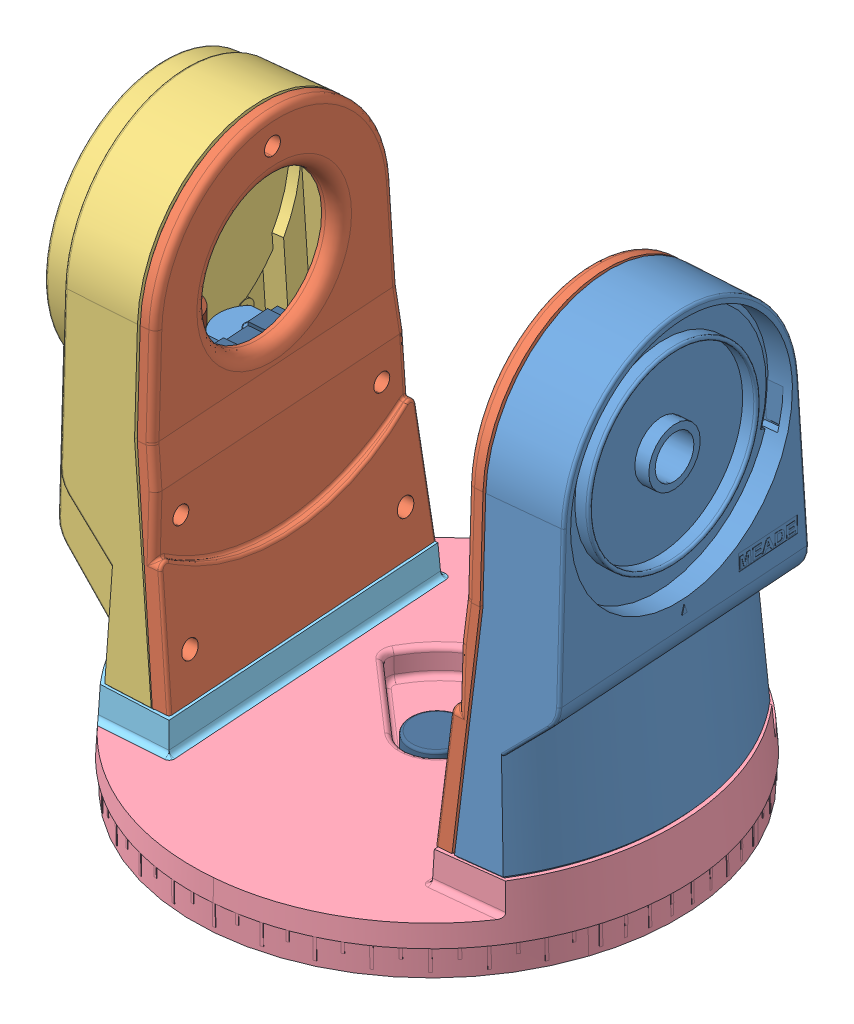
SolidWorks assembly fourche, configuration Défaut. Lengths in mm.
Overall size (198.85 238.33 188.61).
67 component instances, 42 part files, 82 mates.
Components (placement in the parent):
- branche equilibrage-1: branche equilibrage [Défaut] at (-444.0293 45.9192 -837.0232) x (0.999848 0.017413 0.00001) z (0.00001 -0.001172 0.999999) size (42.16 177.75 110.07)
- Plaque carter équilibrage-1: Plaque carter équilibrage [Défaut] at (-443.0317 45.9366 -837.0903) x (0.999848 0.017413 0.00001) z (0.00001 -0.001172 0.999999) size (27.56 165.18 109.18)
- Plaque carter équilibrage-2: Plaque carter équilibrage [Défaut] at (-468.0617 45.0668 -480.7137) x (-0.999848 -0.017413 -0.00001) z (-0.00001 0.001172 -0.999999) size (27.56 165.18 109.18)
- branche motorisée-1: branche motorisée [Défaut] at (-441.716 45.9434 -837.1795) x (0.999848 0.017413 0.00001) z (0.00001 -0.001172 0.999999) size (49.59 177.72 110.04)
- PIED DE fourche-1: PIED DE fourche [Défaut] at (-454.4692 -14.4541 -658.8869) x (0.999848 0.017413 0.00001) z (0.00001 -0.001172 0.999999) size (191.94 35.1 188.57)
  - Pied de fourche-1: Pied de fourche [Défaut] at (12.1809 59.9857 -178.2534) size (191.94 35.1 188.57)
  - Pied de fourche1-1: Pied de fourche1 [Défaut] at (-12.1809 59.9857 178.0188) x (-1 0 0) z (0 0 -1) size (54.8 35.1 115.86)
- rondelle vis m8_50-1: rondelle vis m8_50 [Défaut] at (-454.2843 -25.0712 -659.0167) x (0.997592 0.017452 -0.067129) z (0.017413 -0.999848 -0.001172) size (26.8 26.16 7)
- VisHM8_50-1: VisHM8_50 [Défaut] at (-454.3818 -19.4721 -659.0102) x (0.997592 0.017452 -0.067129) z (0.017413 -0.999848 -0.001172) size (12.6 14.55 55.47)
- limiteur de couple embase-1: limiteur de couple embase [Défaut] at (-453.5008 -70.0544 -659.0694) x (0.06714 0 0.997744) z (-0.997592 -0.017452 0.067129) size (25.3 5 25.3)
- Roue à denture hélicoïdale m=0,5 Z=60-1: Roue à denture hélicoïdale m=0,5 Z=60 [Défaut] at (-453.6431 -61.8856 -659.0599) x (0.201032 0.002353 0.979582) z (-0.017413 0.999848 0.001172) size (31.07 31.07 6.34)
- Levier de débrayage-1: Levier de débrayage [Défaut] at (-491.4971 43.1006 -833.8173) x (0.963244 0.01709 -0.268082) z (0.268062 0.003539 0.963395) size (36.12 10 38.96)
- plateau-1: plateau [Défaut] at (-454.3861 -19.2221 -659.0099) x (-0.997592 -0.017452 0.067129) z (0.017413 -0.999848 -0.001172) size (170 170 47)
- EcrouHM 20-2: EcrouHM 20 [Défaut] at (-453.9456 -44.5183 -659.0395) x (0.06714 0 0.997744) z (-0.017413 0.999848 0.001172) size (30 34.64 12)
- motoreducteur fourche-1: motoreducteur fourche [Défaut] at (-542.1299 45.8782 -641.824) x (0.06714 0 0.997744) z (0.997592 0.017452 -0.067129) size (70.5 139.71 33.06)
  - rep. 01 pignon arbre moteur + disque-1: rep. 01 pignon arbre moteur + disque [Défaut] at (0 -0.36 0) size (19 10.8 19)
  - rep. 02-03 roue Z56-1: rep. 02-03 roue Z56 [Défaut] at (0.8779 -0.6486 0.8082) x (0.995701 0 0.092628) z (-0.092628 0 0.995701) size (28.76 10.95 28.76)
  - rep. 08-09 roue inter-1: rep. 08-09 roue inter [Défaut] at (-0.15 -0.2381 0) x (1 0 0) z (0 0 1) size (12.96 5.74 12.96)
  - rep. 06-07 roue inter-1: rep. 06-07 roue inter [Défaut] at (-0.15 -0.0981 0) x (1 0 0) z (0 0 1) size (13 5.74 13)
  - rep. 04-05 roue inter-1: rep. 04-05 roue inter [Défaut] at (-21.6079 -0.6386 5.1059) x (0.907401 0 -0.420265) z (0.420265 0 0.907401) size (13 5.74 13)
  - bati-1: bati [Défaut] at (103.3128 129.885 -87.3106) size (70.5 138.91 24)
    - Axe Rep19bis-1: Axe Rep19bis [Défaut] at (-92.1856 -130.245 98.2871) x (-0.137137 0 0.990552) z (-0.990552 0 -0.137137) size (3 14 3)
    - moteur-1: moteur [Défaut] at (-103.3128 -129.885 87.3106) size (18 46.5 24)
    - axe-1: axe [Défaut] at (-111.605 -120.0821 97.7106) x (0.934599 0 -0.355704) z (0 -1 0) size (3 3 39)
    - bati2-1: bati2 [Défaut] at (-77.4849 -277.8736 138.6581) x (1 0 0) z (0 0 -1) size (17.4 55.11 17.4)
      - rondelle alu-1: rondelle alu [Défaut] at (-55.9783 -35.2009 30.6529) size (17.4 2.5 17.4)
      - Rondelle M6_1-1: Rondelle M6_1 [Défaut] at (-55.9783 -35.2009 30.6529) size (16.67 2.55 16.67)
      - rondelle alu_1-1: rondelle alu_1 [Défaut] at (-55.9783 -35.2009 30.6529) size (17.4 2.5 17.4)
      - Entretoise_1-1: Entretoise_1 [Défaut] at (-55.9783 -35.2009 30.6529) size (16.5 6 16.5)
      - Entretoise-1: Entretoise [Défaut] at (-55.9783 -35.2009 30.6529) size (16.5 6 16.5)
      - Rondelle M6-1: Rondelle M6 [Défaut] at (-55.9783 -35.2009 30.6529) size (16.67 2.55 16.67)
      - rep. 16 Ecrou M6-1: rep. 16 Ecrou M6 [Défaut] at (18.5294 -120.4752 48.0628) x (-0.896454 0 -0.443136) z (-0.443136 0 0.896454) size (12.68 6 11.39)
    - corps1-1: corps1 [Défaut] at (-126.5989 -147.7633 97.7106) size (62.7 74.5 12)
    - corps2-1: corps2 [Défaut] at (-126.5989 -147.7633 85.7106) size (62.7 50 12) (hidden)
    - châpe en alu-1: châpe en alu [Défaut] at (-133.4632 -157.3984 87.2051) size (33.3 38 19.61)
  - vis-1: vis [Défaut] at (7.3554 -71.4832 9.6533) x (1 0 0) z (0 1 0) size (33.09 33.06 82.71)
    - Vis san fin m=0,5 - 1 filet(s)-2: Vis san fin m=0,5 - 1 filet(s) [Défaut] at (-0.6479 -0.6412 0.3804) x (0.7262 -0.687484 0) z (0 0 1) size (8.16 8.16 68.9)
    - rep12-4: rep12 [Défaut] at (-11.6724 36.0347 43.7266) x (0.537117 -0.843508 0) z (-0.843508 -0.537117 0) size (23.91 29.81 24)
  - engrenage-1: engrenage [Défaut] at (-45.9983 -125.8694 31.0757) x (-0.919401 0 0.393321) z (0.393321 0 0.919401) size (12.99 17.44 12.99)
    - rep.11SLDPRT-1: rep.11SLDPRT [Défaut] at (-64.557 -106.8565 -14.5787) size (9.52 16 9.52)
    - rep. yacine-1: rep. yacine [Défaut] at (-64.557 -106.8565 -14.5787) size (12.99 1.44 12.99)
  - Vis à tête cylindrique à six pans creux Chc M2,5 - 8-1: Vis à tête cylindrique à six pans creux Chc M2,5 - 8 [Défaut] at (6.7074 -20.6971 10.2945) x (0.636786 0 0.771041) z (0 -1 0) size (4.2 4.2 10.57)
  - joint 9 5 emb-1: joint 9 5 emb [Défaut] at (6.7074 -89.1506 10.2945) size (13.5 2 13.5)
  - joint 9 5 emb-2: joint 9 5 emb [Défaut] at (6.7074 -53.1506 10.2945) size (13.5 2 13.5)
- Vis sans tête à six pans creux à bout cuvette M3 - 3-1: Vis sans tête à six pans creux à bout cuvette M3 - 3 [Réaliste] at (-445.1418 -17.1499 -659.6319) x (-0.019293 -0.859815 -0.51024) z (0.066624 -0.510307 0.857408) size (3.03 3.08 3.04)
- Vis à tête cylindrique bombée cruciforme type H M3 - 10-1: Vis à tête cylindrique bombée cruciforme type H M3 - 10 [Filetage Réaliste] at (-521.841 56.7793 -695.504) x (-0.997592 -0.017452 0.067129) z (-0.0364 0.955572 -0.292501) size (12.58 5.6 5.6)
- Vis à tête cylindrique bombée cruciforme type H M3 - 10-2: Vis à tête cylindrique bombée cruciforme type H M3 - 10 [Filetage Réaliste] at (-508.9533 16.8988 -611.179) x (-0.997592 -0.017452 0.067129) z (-0.040277 -0.642181 -0.765494) size (12.58 5.6 5.6)
- Vis à tête cylindrique bombée cruciforme type H M3 - 10-3: Vis à tête cylindrique bombée cruciforme type H M3 - 10 [Filetage Réaliste] at (-514.8616 16.8988 -698.9804) x (-0.997592 -0.017452 0.067129) z (-0.068087 0.06176 -0.995766) size (12.58 5.6 5.6)
- Vis à tête cylindrique bombée cruciforme type H M3 - 10-4: Vis à tête cylindrique bombée cruciforme type H M3 - 10 [Filetage Réaliste] at (-521.2936 154.7556 -654.4481) x (-0.997592 -0.017452 0.067129) z (-0.06714 0 -0.997744) size (12.58 5.6 5.6)
- Vis à tête cylindrique bombée cruciforme type H M3 - 10-5: Vis à tête cylindrique bombée cruciforme type H M3 - 10 [Filetage Réaliste] at (-516.3356 56.7793 -613.689) x (-0.997592 -0.017452 0.067129) z (-0.06714 0 -0.997744) size (12.58 5.6 5.6)
- Vis à tête cylindrique bombée cruciforme type H M3 - 10-7: Vis à tête cylindrique bombée cruciforme type H M3 - 10 [Filetage Réaliste] at (-393.6444 157.0051 -663.0973) x (0.997592 0.017452 -0.067129) z (0.06714 0 0.997744) size (12.58 5.6 5.6)
- Vis à tête cylindrique bombée cruciforme type H M3 - 10-8: Vis à tête cylindrique bombée cruciforme type H M3 - 10 [Filetage Réaliste] at (-401.1787 18.9039 -706.6898) x (0.997592 0.017452 -0.067129) z (0.06714 0 0.997744) size (12.58 5.6 5.6)
- Vis à tête cylindrique bombée cruciforme type H M3 - 10-10: Vis à tête cylindrique bombée cruciforme type H M3 - 10 [Filetage Réaliste] at (-395.1895 59.0113 -704.086) x (0.997592 0.017452 -0.067129) z (0.06714 0 0.997744) size (12.58 5.6 5.6)
- Vis à tête cylindrique fendue CS M4 - 10-1: Vis à tête cylindrique fendue CS M4 - 10 [Défaut] at (-539.7157 125.5672 -628.3483) x (0.067415 -0.016315 0.997592) z (-0.997592 -0.017452 0.067129) size (7 7 10.62)
- Vis à tête cylindrique fendue CS M4 - 10-2: Vis à tête cylindrique fendue CS M4 - 10 [Défaut] at (-538.2089 116.0774 -615.8713) x (0.067415 -0.016315 0.997592) z (-0.997592 -0.017452 0.067129) size (7 7 10.62)
- Vis à tête cylindrique fendue CS M4 - 10-3: Vis à tête cylindrique fendue CS M4 - 10 [Défaut] at (-539.3849 106.5701 -628.3705) x (0.067415 -0.016315 0.997592) z (-0.997592 -0.017452 0.067129) size (7 7 10.62)
- Vis à tête cylindrique bombée cruciforme type H M3 - 12-2: Vis à tête cylindrique bombée cruciforme type H M3 - 12 [Filetage Réaliste] at (-395.2704 18.9039 -618.8883) x (0.997592 0.017452 -0.067129) z (0.067129 0.000586 0.997744) size (14.59 5.6 5.6)
- Vis à tête cylindrique bombée cruciforme type H M3 - 12-3: Vis à tête cylindrique bombée cruciforme type H M3 - 12 [Filetage Réaliste] at (-389.684 59.0113 -622.271) x (0.997592 0.017452 -0.067129) z (0.068185 -0.42423 0.902984) size (14.59 5.6 5.6)
- Vis à tête cylindrique bombée cruciforme type H M3 - 25-1: Vis à tête cylindrique bombée cruciforme type H M3 - 25 [Filetage Réaliste] at (-516.5693 58.6063 -628.1014) x (-0.997592 -0.017452 0.067129) z (-0.067129 0.486457 -0.871122) size (32.61 5.6 5.6)
- Vis à tête cylindrique bombée cruciforme type H M3 - 25-2: Vis à tête cylindrique bombée cruciforme type H M3 - 25 [Filetage Réaliste] at (-520.3322 72.7741 -680.3366) x (-0.997592 -0.017452 0.067129) z (-0.067129 0.486457 -0.871122) size (32.61 5.6 5.6)
- Vis à tête cylindrique bombée cruciforme type H M3 - 25-3: Vis à tête cylindrique bombée cruciforme type H M3 - 25 [Filetage Réaliste] at (-519.8272 43.7786 -680.3706) x (-0.997592 -0.017452 0.067129) z (0.067053 0.00493 0.997737) size (32.61 5.6 5.6)
- Vis à tête cylindrique bombée cruciforme type H M3 - 20-1: Vis à tête cylindrique bombée cruciforme type H M3 - 20 [Filetage Réaliste] at (-531.1265 -25.9655 -653.8459) x (-0.017413 0.999848 0.001172) z (0.998816 0.017342 0.045444) size (22.61 5.6 5.6)
- Vis à tête cylindrique bombée cruciforme type H M3 - 20-2: Vis à tête cylindrique bombée cruciforme type H M3 - 20 [Filetage Réaliste] at (-512.8439 -25.695 -612.9812) x (-0.017413 0.999848 0.001172) z (0.998816 0.017342 0.045444) size (22.61 5.6 5.6)
- Vis à tête cylindrique bombée cruciforme type H M3 - 20-3: Vis à tête cylindrique bombée cruciforme type H M3 - 20 [Filetage Réaliste] at (-517.7505 -25.6821 -696.841) x (-0.017413 0.999848 0.001172) z (0.998816 0.017342 0.045444) size (22.61 5.6 5.6)
- Vis à tête cylindrique bombée cruciforme type H M3 - 20-4: Vis à tête cylindrique bombée cruciforme type H M3 - 20 [Filetage Réaliste] at (-395.7403 -23.5476 -705.0512) x (-0.017413 0.999848 0.001172) z (0.998816 0.017342 0.045444) size (22.61 5.6 5.6)
- Vis à tête cylindrique bombée cruciforme type H M3 - 20-5: Vis à tête cylindrique bombée cruciforme type H M3 - 20 [Filetage Réaliste] at (-377.4577 -23.2771 -664.1865) x (-0.017413 0.999848 0.001172) z (0.998816 0.017342 0.045444) size (22.61 5.6 5.6)
- Vis à tête cylindrique bombée cruciforme type H M3 - 20-6: Vis à tête cylindrique bombée cruciforme type H M3 - 20 [Filetage Réaliste] at (-390.8337 -23.5604 -621.1914) x (-0.017413 0.999848 0.001172) z (0.998816 0.017342 0.045444) size (22.61 5.6 5.6)
Mates (geometry in assembly coordinates):
- Coïncidente2: coincident anti-aligned: plane of branche equilibrage-1 through (-369.0099 3.4762 -719.0226) normal (0.034821 -0.999391 -0.002343); plane of PIED DE fourche-1/Pied de fourche-1 through (-361.0465 3.5004 -611.0232) normal (-0.034821 0.999391 0.002343)
- Coaxiale4: concentric anti-aligned: cylinder of branche equilibrage-1 through (-391.0008 157.0513 -663.2752) axis (-0.997592 -0.017452 0.067129) radius 1.25; cylinder of Plaque carter équilibrage-1 through (-402.4136 156.8517 -662.5072) axis (0.997592 0.017452 -0.067129) radius 1.5
- Coïncidente10: coincident anti-aligned: plane of branche equilibrage-1 through (-397.0052 121.4404 -709.6249) normal (-0.997592 -0.017452 0.067129); plane of Plaque carter équilibrage-1 through (-408.418 121.5329 -879.2025) normal (0.997592 0.017452 -0.067129)
- Parallèle1: parallel aligned: plane of branche equilibrage-1 through (-369.0099 3.4762 -719.0226) normal (0.034821 -0.999391 -0.002343); plane of Plaque carter équilibrage-1 through (-422.1214 1.9816 -878.2804) normal (0.034821 -0.999391 -0.002343)
- Coaxiale9: concentric anti-aligned: cone of Plaque carter équilibrage-2 through (-509.6865 154.9588 -655.2893) axis (-0.997592 -0.017452 0.067129); cylinder of branche motorisée-1 through (-524.1906 154.705 -654.3133) axis (0.997592 0.017452 -0.067129) radius 1.25
- Coïncidente13: coincident anti-aligned: plane of Plaque carter équilibrage-2 through (-505.285 119.3131 -438.4259) normal (-0.997592 -0.017452 0.067129); plane of branche motorisée-1 through (-516.6997 119.2197 -608.081) normal (0.997592 0.017452 -0.067129)
- Coïncidente21: coincident: line of Plaque carter équilibrage-1 through (-403.9093 2.9849 -608.7792) axis (-0.06714 0 -0.997744); plane of PIED DE fourche-1/Pied de fourche-1 through (-403.8836 2.0012 -608.1406) normal (-0.997592 0.017452 0.067129)
- Coïncidente30: coincident: plane of Plaque carter équilibrage-1; line of PIED DE fourche-1/Pied de fourche1-1 through (-454.3978 -18.553 -659.0091) axis (0.017413 -0.999848 -0.001172)
- Coïncidente34: coincident: line of Plaque carter équilibrage-2 through (-679.7698 -1.6347 -696.1892) axis (0.067167 -0.001579 0.99774); plane of PIED DE fourche-1/Pied de fourche1-1 through (-505.5991 0.3489 -709.8313) normal (0.996376 0.052336 -0.067048)
- Coaxiale10: concentric anti-aligned: cylinder of rondelle vis m8_50-1 through (-454.2599 -26.471 -659.0184) axis (-0.017413 0.999848 0.001172) radius 4.1; cylinder of VisHM8_50-1 through (-454.3818 -19.4721 -659.0102) axis (0.017413 -0.999848 -0.001172) radius 4
- Coaxiale11: concentric aligned: cylinder of PIED DE fourche-1/Pied de fourche-1 through (-454.4758 -14.0729 -659.0038) axis (0.017413 -0.999848 -0.001172) radius 5.4; cylinder of VisHM8_50-1 through (-454.3818 -19.4721 -659.0102) axis (0.017413 -0.999848 -0.001172) radius 4
- Coïncidente52: coincident anti-aligned: plane of rondelle vis m8_50-1 through (-454.3818 -19.4721 -659.0102) normal (-0.017413 0.999848 0.001172); plane of VisHM8_50-1 through (-447.8527 -19.3621 -655.804) normal (0.017413 -0.999848 -0.001172)
- Parallèle2: parallel aligned: plane of rondelle vis m8_50-1 through (-450.1698 -26.3995 -659.2936) normal (-0.997592 -0.017452 0.067129); plane of VisHM8_50-1 through (-450.6882 -24.4364 -635.2044) normal (-0.997592 -0.017452 0.067129)
- Coïncidente54: coincident anti-aligned: plane of PIED DE fourche-1/Pied de fourche-1 through (-454.2843 -25.0712 -659.0167) normal (0.017413 -0.999848 -0.001172); plane of rondelle vis m8_50-1 through (-454.2843 -25.0712 -659.0167) normal (-0.017413 0.999848 0.001172)
- Parallèle3: parallel: line of PIED DE fourche-1/Pied de fourche1-1 through (-497.7587 -8.9641 -600.586) axis (-0.06714 0 -0.997744); plane of rondelle vis m8_50-1 through (-458.35 -26.5426 -658.7431) normal (0.997592 0.017452 -0.067129)
- Coïncidente56: coincident anti-aligned: plane of Levier de débrayage-1 through (-454.3713 -20.072 -659.0109) normal (0.017413 -0.999848 -0.001172); plane of PIED DE fourche-1/Pied de fourche-1 through (-425.2551 -19.5401 -680.176) normal (-0.017413 0.999848 0.001172)
- Parallèle4: parallel anti-aligned: plane of VisHM8_50-1 through (-454.9625 -14.1729 -666.2621) normal (0.440651 0.008726 -0.897636); plane of Levier de débrayage-1 through (-455.3417 6.7117 -666.4681) normal (-0.440651 -0.008726 0.897636)
- Coïncidente61: coincident anti-aligned: plane of limiteur de couple embase-1 through (-454.4372 -65.0551 -671.685) normal (-0.017413 0.999848 0.001172); plane of Roue à denture hélicoïdale m=0,5 Z=60-1 through (-453.5879 -65.0551 -659.0636) normal (0.017413 -0.999848 -0.001172)
- Coaxiale20: concentric aligned: cylinder of limiteur de couple embase-1 through (-453.5008 -70.0544 -659.0694) axis (0.017413 -0.999848 -0.001172) radius 12.65; cylinder of Roue à denture hélicoïdale m=0,5 Z=60-1 through (-453.6983 -58.7161 -659.0561) axis (0.017413 -0.999848 -0.001172) radius 6.85
- Coaxiale21: concentric aligned: cylinder of VisHM8_50-1 through (-454.3818 -19.4721 -659.0102) axis (0.017413 -0.999848 -0.001172) radius 4; cylinder of limiteur de couple embase-1 through (-453.5008 -70.0544 -659.0694) axis (0.017413 -0.999848 -0.001172) radius 3.4
- Coaxiale22: concentric anti-aligned: cylinder of VisHM8_50-1 through (-454.3818 -19.4721 -659.0102) axis (0.017413 -0.999848 -0.001172) radius 4; cylinder of plateau-1 through (-454.3339 -22.2217 -659.0134) axis (-0.017413 0.999848 0.001172) radius 85
- Distance1: distance = 1 mm anti-aligned: plane of plateau-1 through (-454.441 -16.0726 -659.0062) normal (-0.017413 0.999848 0.001172); plane of PIED DE fourche-1/Pied de fourche-1 through (-377.624 -13.7286 -664.1753) normal (0.017413 -0.999848 -0.001172)
- Coïncidente64: coincident aligned: plane of PIED DE fourche-1/Pied de fourche-1; plane of plateau-1
- Parallèle5: parallel anti-aligned: plane of limiteur de couple embase-1 through (-441.0163 -66.7384 -657.4039) normal (-0.06714 0 -0.997744); plane of plateau-1 through (-456.7222 -64.2727 -656.3721) normal (0.06714 0 0.997744)
- Parallèle9: parallel anti-aligned: plane of branche motorisée-1 through (-539.5714 0.3489 -599.0106) normal (0 -1 0); plane of PIED DE fourche-1/Pied de fourche1-1 through (-548.4623 0.3489 -706.947) normal (0 1 0)
- Coïncidente80: coincident: point of branche motorisée-1; line of PIED DE fourche-1/Pied de fourche1-1 through (-531.345 -13.4174 -653.8312) axis (0.017413 -0.999848 -0.001172)
- Coaxiale35: concentric anti-aligned: cylinder of VisHM8_50-1 through (-454.3818 -19.4721 -659.0102) axis (0.017413 -0.999848 -0.001172) radius 4; cone of Levier de débrayage-1 through (-454.5455 -10.0735 -658.9991) axis (-0.017413 0.999848 0.001172)
- Coïncidente82: coincident anti-aligned: plane of rondelle vis m8_50-1 through (-454.2599 -26.471 -659.0184) normal (0.017413 -0.999848 -0.001172); plane of plateau-1 through (-454.2599 -26.471 -659.0184) normal (-0.017413 0.999848 0.001172)
- Coïncidente83: coincident anti-aligned: plane of Roue à denture hélicoïdale m=0,5 Z=60-1 through (-453.6983 -58.7161 -659.0561) normal (-0.017413 0.999848 0.001172); plane of plateau-1 through (-453.6983 -58.7161 -659.0561) normal (0.017413 -0.999848 -0.001172)
- Parallèle11: parallel aligned: line of Plaque carter équilibrage-2 through (-505.674 1.314 -709.1265) axis (0.06714 0 0.997744); line of PIED DE fourche-1/Pied de fourche1-1 through (-505.6487 0.3489 -710.5673) axis (0.06714 0 0.997744)
- Coaxiale23: concentric anti-aligned: cylinder of VisHM8_50-1 through (-454.3818 -19.4721 -659.0102) axis (0.017413 -0.999848 -0.001172) radius 4; cylinder of EcrouHM 20-2 through (-453.7366 -56.5164 -659.0536) axis (-0.017413 0.999848 0.001172) radius 10
- Perpendiculaire1: perpendicular: plane of Plaque carter équilibrage-2 through (-510.8056 116.9333 -655.1538) normal (0.997592 0.017452 -0.067129); plane of EcrouHM 20-2 through (-461.3689 -56.6676 -643.5061) normal (0.06714 0 0.997744)
- Parallèle12: parallel anti-aligned: plane of plateau-1 through (-454.3339 -22.2217 -659.0134) normal (0.017413 -0.999848 -0.001172); plane of motoreducteur fourche-1/bati-1/châpe en alu-1 through (-541.8121 135.0238 -621.2916) normal (-0.017413 0.999848 0.001172)
- Coaxiale16: concentric anti-aligned: cylinder of branche motorisée-1 through (-542.1099 125.5253 -628.1871) axis (0.997592 0.017452 -0.067129) radius 1.25; cylinder of motoreducteur fourche-1/bati-1/châpe en alu-1 through (-522.5571 125.8673 -629.5029) axis (-0.997592 -0.017452 0.067129) radius 2.15
- Coïncidente99: coincident anti-aligned: plane of branche motorisée-1 through (-541.7791 106.5282 -628.2094) normal (0.997592 0.017452 -0.067129); plane of motoreducteur fourche-1/bati-1/châpe en alu-1 through (-541.4391 97.0296 -625.6264) normal (-0.997592 -0.017452 0.067129)
- Coaxiale15: concentric anti-aligned: cylinder of Levier de débrayage-1 through (-447.935 -17.1987 -659.444) axis (-0.997592 -0.017452 0.067129) radius 1.25; cylinder of Vis sans tête à six pans creux à bout cuvette M3 - 3-1 through (-445.1418 -17.1499 -659.6319) axis (0.997592 0.017452 -0.067129) radius 1.5
- Coïncidente97: coincident aligned: plane of VisHM8_50-1 through (-448.4334 -14.0629 -663.056) normal (0.997592 0.017452 -0.067129); circle of Vis sans tête à six pans creux à bout cuvette M3 - 3-1
- Coaxiale36: concentric anti-aligned: cone of Plaque carter équilibrage-2 through (-510.7287 56.9737 -696.2517) axis (-0.997592 -0.017452 0.067129); cylinder of Vis à tête cylindrique bombée cruciforme type H M3 - 10-1 through (-521.841 56.7793 -695.504) axis (0.997592 0.017452 -0.067129) radius 2.8
- Coïncidente107: coincident anti-aligned: plane of Plaque carter équilibrage-2 through (-524.0736 54.2581 -693.5848) normal (0.997592 0.017452 -0.067129); plane of Vis à tête cylindrique bombée cruciforme type H M3 - 10-1 through (-524.2353 56.7374 -695.3428) normal (-0.997592 -0.017452 0.067129)
- Coaxiale37: concentric anti-aligned: cone of Plaque carter équilibrage-2 through (-500.5661 17.0456 -611.7433) axis (-0.997592 -0.017452 0.067129); cylinder of Vis à tête cylindrique bombée cruciforme type H M3 - 10-2 through (-508.9533 16.8988 -611.179) axis (0.997592 0.017452 -0.067129) radius 2.8
- Coïncidente106: coincident anti-aligned: plane of Plaque carter équilibrage-2 through (-511.1798 14.2852 -609.1943) normal (0.997592 0.017452 -0.067129); plane of Vis à tête cylindrique bombée cruciforme type H M3 - 10-2 through (-511.3475 16.8569 -611.0178) normal (-0.997592 -0.017452 0.067129)
- Coaxiale19: concentric anti-aligned: cone of Plaque carter équilibrage-2 through (-506.4744 17.0456 -699.5448) axis (-0.997592 -0.017452 0.067129); cylinder of Vis à tête cylindrique bombée cruciforme type H M3 - 10-3 through (-514.8616 16.8988 -698.9804) axis (0.997592 0.017452 -0.067129) radius 2.8
- Coïncidente102: coincident anti-aligned: plane of Plaque carter équilibrage-2 through (-517.0881 14.2852 -696.9958) normal (0.997592 0.017452 -0.067129); plane of Vis à tête cylindrique bombée cruciforme type H M3 - 10-3 through (-517.2558 16.8569 -698.8193) normal (-0.997592 -0.017452 0.067129)
- Coïncidente108: coincident anti-aligned: plane of Plaque carter équilibrage-2 through (-523.7885 154.7138 -655.7836) normal (0.997592 0.017452 -0.067129); plane of Vis à tête cylindrique bombée cruciforme type H M3 - 10-4 through (-523.6878 154.7138 -654.287) normal (-0.997592 -0.017452 0.067129)
- Coaxiale38: concentric anti-aligned: cone of Plaque carter équilibrage-2 through (-523.6878 154.7138 -654.287) axis (-0.997592 -0.017452 0.067129); cylinder of Vis à tête cylindrique bombée cruciforme type H M3 - 10-4 through (-521.2936 154.7556 -654.4481) axis (0.997592 0.017452 -0.067129) radius 2.8
- Coaxiale24: concentric anti-aligned: cone of Plaque carter équilibrage-2 through (-505.2232 56.9737 -614.4367) axis (-0.997592 -0.017452 0.067129); cylinder of Vis à tête cylindrique bombée cruciforme type H M3 - 10-5 through (-516.3356 56.7793 -613.689) axis (0.997592 0.017452 -0.067129) radius 2.8
- Coïncidente109: coincident anti-aligned: plane of Plaque carter équilibrage-2 through (-518.8051 54.2581 -615.2917) normal (0.997592 0.017452 -0.067129); plane of Vis à tête cylindrique bombée cruciforme type H M3 - 10-5 through (-518.7298 56.7374 -613.5279) normal (-0.997592 -0.017452 0.067129)
- Coaxiale29: concentric anti-aligned: cone of Plaque carter équilibrage-1 through (-391.2502 157.047 -663.2584) axis (0.997592 0.017452 -0.067129); cylinder of Vis à tête cylindrique bombée cruciforme type H M3 - 10-7 through (-393.6444 157.0051 -663.0973) axis (-0.997592 -0.017452 0.067129) radius 2.8
- Coïncidente114: coincident anti-aligned: plane of Plaque carter équilibrage-1 through (-391.1495 157.047 -661.7618) normal (-0.997592 -0.017452 0.067129); plane of Vis à tête cylindrique bombée cruciforme type H M3 - 10-7 through (-391.2502 157.047 -663.2584) normal (0.997592 0.017452 -0.067129)
- Coïncidente111: coincident anti-aligned: plane of Plaque carter équilibrage-1 through (-398.8626 16.3741 -708.6804) normal (-0.997592 -0.017452 0.067129); plane of Vis à tête cylindrique bombée cruciforme type H M3 - 10-8 through (-398.7845 18.9458 -706.8509) normal (0.997592 0.017452 -0.067129)
- Coaxiale26: concentric anti-aligned: cone of Plaque carter équilibrage-1 through (-409.566 18.7572 -706.1254) axis (0.997592 0.017452 -0.067129); cylinder of Vis à tête cylindrique bombée cruciforme type H M3 - 10-8 through (-401.1787 18.9039 -706.6898) axis (-0.997592 -0.017452 0.067129) radius 2.8
- Coaxiale25: concentric anti-aligned: cone of Plaque carter équilibrage-1 through (-406.3018 58.8169 -703.3382) axis (0.997592 0.017452 -0.067129); cylinder of Vis à tête cylindrique bombée cruciforme type H M3 - 10-10 through (-395.1895 59.0113 -704.086) axis (-0.997592 -0.017452 0.067129) radius 2.8
- Coïncidente110: coincident anti-aligned: plane of Plaque carter équilibrage-1 through (-392.6336 56.5738 -702.4891) normal (-0.997592 -0.017452 0.067129); plane of Vis à tête cylindrique bombée cruciforme type H M3 - 10-10 through (-392.7953 59.0532 -704.2471) normal (0.997592 0.017452 -0.067129)
- Coaxiale39: concentric anti-aligned: cylinder of branche motorisée-1 through (-541.1019 116.0267 -615.6766) axis (0.997592 0.017452 -0.067129) radius 1.25; cylinder of Vis à tête cylindrique fendue CS M4 - 10-2 through (-538.2089 116.0774 -615.8713) axis (-0.997592 -0.017452 0.067129) radius 2
- Coïncidente115: coincident anti-aligned: plane of motoreducteur fourche-1/bati-1/châpe en alu-1 through (-536.8565 116.0773 -595.7741) normal (0.997592 0.017452 -0.067129); plane of Vis à tête cylindrique fendue CS M4 - 10-2 through (-538.2089 116.0774 -615.8713) normal (-0.997592 -0.017452 0.067129)
- Coïncidente116: coincident aligned: plane of Vis à tête cylindrique fendue CS M4 - 10-1 through (-539.7157 125.5672 -628.3483) normal (-0.997592 -0.017452 0.067129); plane of Vis à tête cylindrique fendue CS M4 - 10-3 through (-539.3849 106.5701 -628.3705) normal (-0.997592 -0.017452 0.067129)
- Coaxiale40: concentric anti-aligned: cylinder of branche motorisée-1 through (-542.1099 125.5253 -628.1871) axis (0.997592 0.017452 -0.067129) radius 1.25; cylinder of Vis à tête cylindrique fendue CS M4 - 10-1 through (-539.7157 125.5672 -628.3483) axis (-0.997592 -0.017452 0.067129) radius 2
- Coaxiale41: concentric anti-aligned: cylinder of branche motorisée-1 through (-541.7791 106.5282 -628.2094) axis (0.997592 0.017452 -0.067129) radius 1.25; cylinder of Vis à tête cylindrique fendue CS M4 - 10-3 through (-539.3849 106.5701 -628.3705) axis (-0.997592 -0.017452 0.067129) radius 2
- Coïncidente117: coincident anti-aligned: plane of motoreducteur fourche-1/bati-1/châpe en alu-1 through (-539.7832 102.0707 -635.4598) normal (0.997592 0.017452 -0.067129); plane of Vis à tête cylindrique fendue CS M4 - 10-1 through (-539.7157 125.5672 -628.3483) normal (-0.997592 -0.017452 0.067129)
- Coaxiale43: concentric anti-aligned: cylinder of motoreducteur fourche-1/bati-1/corps1-1 through (-518.9635 58.5644 -627.9402) axis (-0.997592 -0.017452 0.067129) radius 1.75; cylinder of Vis à tête cylindrique bombée cruciforme type H M3 - 25-1 through (-516.5693 58.6063 -628.1014) axis (0.997592 0.017452 -0.067129) radius 2.8
- Coïncidente119: coincident anti-aligned: plane of motoreducteur fourche-1/bati-1/corps1-1 through (-522.7264 72.7323 -680.1755) normal (0.997592 0.017452 -0.067129); plane of Vis à tête cylindrique bombée cruciforme type H M3 - 25-1 through (-518.9635 58.5644 -627.9402) normal (-0.997592 -0.017452 0.067129)
- Coaxiale44: concentric anti-aligned: cylinder of motoreducteur fourche-1/bati-1/corps1-1 through (-522.2214 43.7367 -680.2095) axis (-0.997592 -0.017452 0.067129) radius 1.75; cylinder of Vis à tête cylindrique bombée cruciforme type H M3 - 25-3 through (-519.8272 43.7786 -680.3706) axis (0.997592 0.017452 -0.067129) radius 2.8
- Coïncidente120: coincident anti-aligned: plane of motoreducteur fourche-1/bati-1/corps1-1 through (-522.7264 72.7323 -680.1755) normal (0.997592 0.017452 -0.067129); plane of Vis à tête cylindrique bombée cruciforme type H M3 - 25-3 through (-522.2214 43.7367 -680.2095) normal (-0.997592 -0.017452 0.067129)
- Coaxiale45: concentric anti-aligned: cylinder of Vis à tête cylindrique bombée cruciforme type H M3 - 25-2 through (-520.3322 72.7741 -680.3366) axis (0.997592 0.017452 -0.067129) radius 2.8; cylinder of motoreducteur fourche-1/bati-1/corps1-1 through (-522.7264 72.7323 -680.1755) axis (-0.997592 -0.017452 0.067129) radius 1.15
- Coïncidente121: coincident anti-aligned: plane of motoreducteur fourche-1/bati-1/corps1-1 through (-522.7264 72.7323 -680.1755) normal (0.997592 0.017452 -0.067129); plane of Vis à tête cylindrique bombée cruciforme type H M3 - 25-2 through (-522.7264 72.7323 -680.1755) normal (-0.997592 -0.017452 0.067129)
- Coaxiale48: concentric anti-aligned: cone of Plaque carter équilibrage-1 through (-400.7964 58.8169 -621.5233) axis (0.997592 0.017452 -0.067129); cylinder of Vis à tête cylindrique bombée cruciforme type H M3 - 12-3 through (-389.684 59.0113 -622.271) axis (-0.997592 -0.017452 0.067129) radius 2.8
- Coïncidente122: coincident anti-aligned: plane of Plaque carter équilibrage-1 through (-387.3651 56.5738 -624.196) normal (-0.997592 -0.017452 0.067129); plane of Vis à tête cylindrique bombée cruciforme type H M3 - 12-3 through (-387.2898 59.0532 -622.4322) normal (0.997592 0.017452 -0.067129)
- Coaxiale49: concentric anti-aligned: cone of Plaque carter équilibrage-1 through (-403.6577 18.7572 -618.3239) axis (0.997592 0.017452 -0.067129); cylinder of Vis à tête cylindrique bombée cruciforme type H M3 - 12-2 through (-395.2704 18.9039 -618.8883) axis (-0.997592 -0.017452 0.067129) radius 2.8
- Coïncidente123: coincident anti-aligned: plane of Plaque carter équilibrage-1 through (-392.9543 16.3741 -620.879) normal (-0.997592 -0.017452 0.067129); plane of Vis à tête cylindrique bombée cruciforme type H M3 - 12-2 through (-392.8762 18.9458 -619.0494) normal (0.997592 0.017452 -0.067129)
- Coïncidente124: coincident anti-aligned: plane of branche motorisée-1 through (-539.5714 0.3489 -599.0106) normal (0 -1 0); plane of PIED DE fourche-1/Pied de fourche1-1 through (-548.4623 0.3489 -706.947) normal (0 1 0)
- Coïncidente125: coincident anti-aligned: plane of plateau-1 through (-454.3339 -22.2217 -659.0134) normal (0.017413 -0.999848 -0.001172); plane of Vis à tête cylindrique bombée cruciforme type H M3 - 20-1 through (-531.1682 -23.5658 -653.8431) normal (-0.017413 0.999848 0.001172)
- Coaxiale31: concentric aligned: cylinder of plateau-1 through (-531.1682 -23.5658 -653.8431) axis (0.017413 -0.999848 -0.001172) radius 1.7; cylinder of Vis à tête cylindrique bombée cruciforme type H M3 - 20-1 through (-531.1265 -25.9655 -653.8459) axis (0.017413 -0.999848 -0.001172) radius 2.8
- Coaxiale30: concentric aligned: cylinder of plateau-1 through (-512.8857 -23.2953 -612.9784) axis (0.017413 -0.999848 -0.001172) radius 1.7; cylinder of Vis à tête cylindrique bombée cruciforme type H M3 - 20-2 through (-512.8439 -25.695 -612.9812) axis (0.017413 -0.999848 -0.001172) radius 2.8
- Coïncidente126: coincident anti-aligned: plane of plateau-1 through (-454.3339 -22.2217 -659.0134) normal (0.017413 -0.999848 -0.001172); plane of Vis à tête cylindrique bombée cruciforme type H M3 - 20-2 through (-512.8857 -23.2953 -612.9784) normal (-0.017413 0.999848 0.001172)
- Coïncidente118: coincident anti-aligned: plane of plateau-1 through (-454.3339 -22.2217 -659.0134) normal (0.017413 -0.999848 -0.001172); plane of Vis à tête cylindrique bombée cruciforme type H M3 - 20-3 through (-517.7923 -23.2825 -696.8381) normal (-0.017413 0.999848 0.001172)
- Coaxiale32: concentric aligned: cylinder of plateau-1 through (-517.7923 -23.2825 -696.8381) axis (0.017413 -0.999848 -0.001172) radius 1.7; cylinder of Vis à tête cylindrique bombée cruciforme type H M3 - 20-3 through (-517.7505 -25.6821 -696.841) axis (0.017413 -0.999848 -0.001172) radius 2.8
- Coïncidente127: coincident anti-aligned: plane of plateau-1 through (-454.3339 -22.2217 -659.0134) normal (0.017413 -0.999848 -0.001172); plane of Vis à tête cylindrique bombée cruciforme type H M3 - 20-4 through (-395.7821 -21.148 -705.0484) normal (-0.017413 0.999848 0.001172)
- Coaxiale33: concentric aligned: cylinder of plateau-1 through (-395.7821 -21.148 -705.0484) axis (0.017413 -0.999848 -0.001172) radius 1.7; cylinder of Vis à tête cylindrique bombée cruciforme type H M3 - 20-4 through (-395.7403 -23.5476 -705.0512) axis (0.017413 -0.999848 -0.001172) radius 2.8
- Coïncidente128: coincident anti-aligned: plane of plateau-1 through (-454.3339 -22.2217 -659.0134) normal (0.017413 -0.999848 -0.001172); plane of Vis à tête cylindrique bombée cruciforme type H M3 - 20-5 through (-377.4995 -20.8775 -664.1837) normal (-0.017413 0.999848 0.001172)
- Coaxiale34: concentric aligned: cylinder of plateau-1 through (-377.4995 -20.8775 -664.1837) axis (0.017413 -0.999848 -0.001172) radius 1.7; cylinder of Vis à tête cylindrique bombée cruciforme type H M3 - 20-5 through (-377.4577 -23.2771 -664.1865) axis (0.017413 -0.999848 -0.001172) radius 2.8
- Coïncidente129: coincident anti-aligned: plane of plateau-1 through (-454.3339 -22.2217 -659.0134) normal (0.017413 -0.999848 -0.001172); plane of Vis à tête cylindrique bombée cruciforme type H M3 - 20-6 through (-390.8755 -21.1608 -621.1886) normal (-0.017413 0.999848 0.001172)
- Coaxiale50: concentric aligned: cylinder of plateau-1 through (-390.8755 -21.1608 -621.1886) axis (0.017413 -0.999848 -0.001172) radius 1.7; cylinder of Vis à tête cylindrique bombée cruciforme type H M3 - 20-6 through (-390.8337 -23.5604 -621.1914) axis (0.017413 -0.999848 -0.001172) radius 2.8
